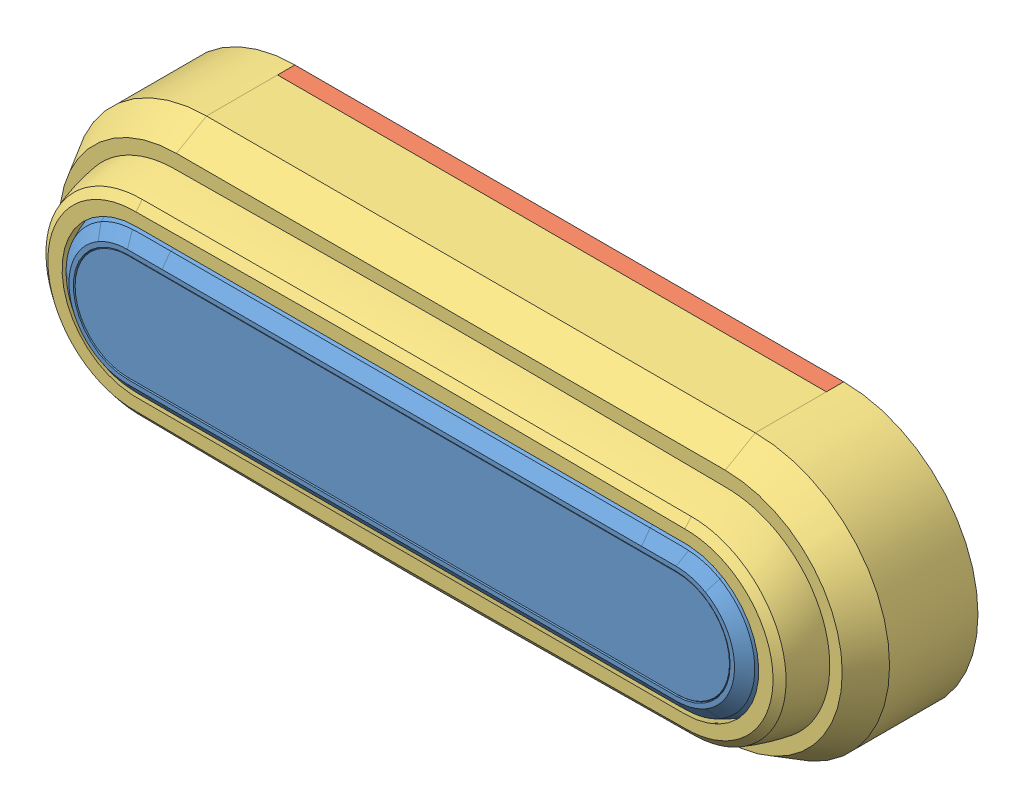
SolidWorks assembly Intel_RealSense_D455, configuration Default. Lengths in mm.
Overall size (141.5 46.5 29.01).
3 component instances, 3 part files, 5 mates.
Components (placement in the parent):
- Intel Realsense D455-1: Intel Realsense D455 [Default] at origin
- Blocco D455-1: Blocco D455 [Default] at (0 0 -29) x (0 -1 0) z (0 0 1)
- Cover Telecamera-1: Cover Telecamera [Default] at (0 0 -1.5) x (0 -1 0) z (0 0 1)
Mates (geometry in assembly coordinates):
- Coincident1: coordinate: point of Intel Realsense D455-1
- Coincident3: coincident aligned: plane of Cover Telecamera-1 through (0 0 -1.5) normal (1 0 0)
- Coincident4: coincident anti-aligned: plane of Blocco D455-1 through (-47.5 0 -26) normal (0 0 1); plane of Cover Telecamera-1 through (47.5 0 -26) normal (0 0 -1)
- Coincident5: coincident aligned: plane of Blocco D455-1 through (0 0 -29) normal (1 0 0)
- Coincident6: coincident anti-aligned: plane of Intel Realsense D455-1 through (0 0 -26) normal (0 0 -1); plane of Blocco D455-1 through (-47.5 0 -26) normal (0 0 1)
